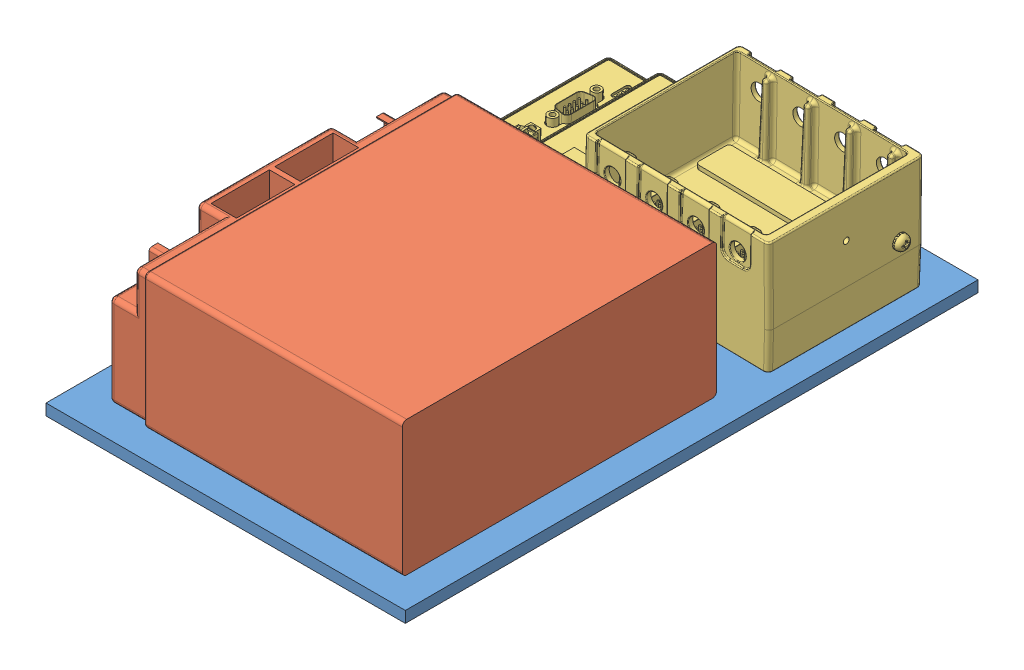
SolidWorks assembly cRio and Battery, configuration Default. Lengths in mm.
Overall size (203.2 82.55 323.85).
3 component instances, 3 part files, 3 mates.
Components (placement in the parent):
- cRIO and Battery Base-1: cRIO and Battery Base [Default] at (-76.8047 3.0824 116.7528) size (203.2 6.35 323.85)
- Battery1-1: Battery1 [Default] at (79.8759 71.6456 0.1884) x (0 0 1) z (-1 0 0) size (177.8 76.2 167.13)
- User Library-cu_crio-frcII_4-slot_-2: User Library-cu_crio-frcII_4-slot_ [Default] at (11.8638 10.7688 -101.5676) x (0 0.000242 1) z (-0.999848 0.017452 -0.000004) size (89.5 64.8 182.23)
Mates (geometry in assembly coordinates):
- Coincident1: coincident anti-aligned: plane of cRIO and Battery Base-1 through (-76.8047 9.4324 116.7528) normal (0 1 0); plane of Battery1-1 through (79.8759 9.4324 0.1884) normal (0 -1 0)
- Distance4: distance = 19.05 mm aligned: plane of Battery1-1 through (-87.2561 71.6456 0.1884) normal (-1 0 0); plane of cRIO and Battery Base-1 through (-106.3061 9.4324 -163.6928) normal (-1 0 0)
- Distance7: distance = 12.7 mm aligned: plane of User Library-cu_crio-frcII_4-slot_-2 through (-93.6061 12.5989 -146.4447) normal (-1 0 0); plane of cRIO and Battery Base-1 through (-106.3061 9.4324 -163.6928) normal (-1 0 0)
